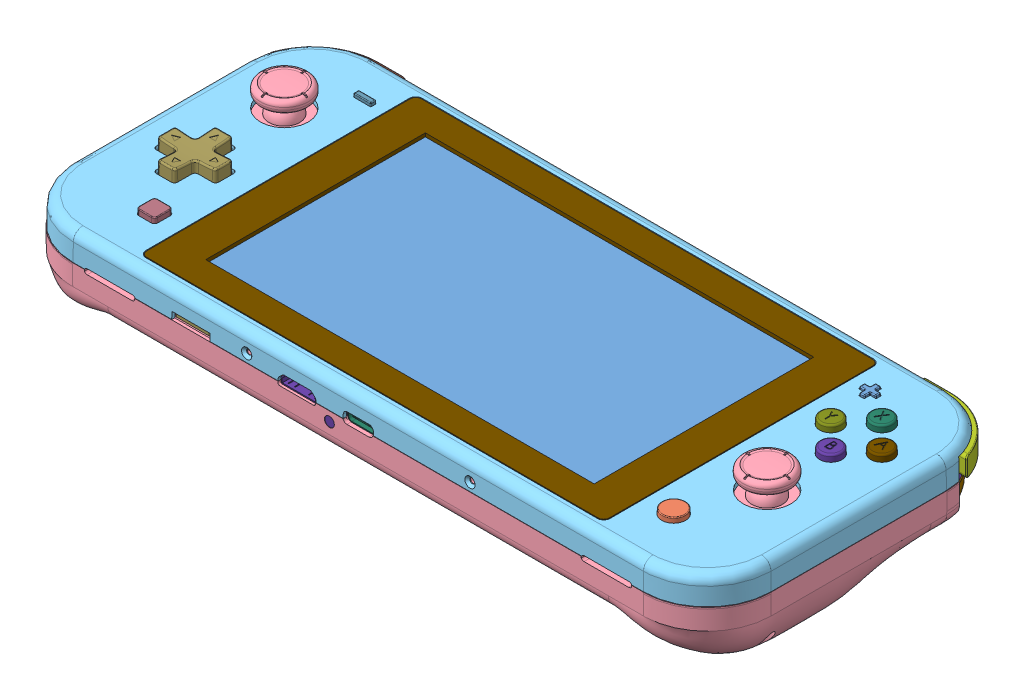
SolidWorks assembly Assembly Retro Lite CM5_1, configuration Default. Lengths in mm. (continued)
Components (placement in the parent): (continued)
- Switch Lite D-Pad_1-1: Switch Lite D-Pad_1 [Default] at (-86.4992 8.2269 18.5) size (20.6 9.05 20.6)
- Select_Button_1-1: Select_Button_1 [Default] at (-1.1992 10.6269 0) size (9.88 4.75 9.88)
- Minus Button_1-1: Minus Button_1 [Default] at (-93.2142 14.0269 -94.6231) x (0 0 -1) z (1 0 0) size (5.72 4.5 9.47)
- NuckDeck X_1-1: NuckDeck X_1 [Default] at (89.6642 6.7269 -27) size (9.68 5.75 9.89)
- NuckDeck Y_1-1: NuckDeck Y_1 [Default] at (81.6642 6.2269 -19) size (9.68 5.75 9.89)
- NuckDeck B_1-1: NuckDeck B_1 [Default] at (89.6642 6.7269 -11) size (9.68 5.75 9.89)
- NuckDeck A_1-1: NuckDeck A_1 [Default] at (97.6642 7.2269 -19) size (9.68 5.75 9.89)
- Plus_Button_1-1: Plus_Button_1 [Default] at (1.1992 9.5269 0) size (5.18 4.7 5.18)
- Start_Button_1-1: Start_Button_1 [Default] at (55.5311 21.0456 -12.0161) x (0 -1 0) z (0 0 1) size (5.05 11.38 11.38)
- Power-Volume Button-On_Off-1: Power-Volume Button-On_Off [Default] at (52.5142 1.7499 -46.5415) x (-1 0 0) z (0 -1 0) size (9.02 8.15 5.02)
- Switch Lite Fan_1-1: Switch Lite Fan_1 [Default] at (-39.8893 -3 21.8439) x (-1 0 0) z (0 0 1) size (44.11 7.2 36.36)
- Case Front_2-1: Case Front_2 [Default] at origin size (219.25 9 95.96)
- Volume Buttons-1: Volume Buttons [Default] at (0.7169 -0.25 -2.25) size (13.02 5.02 8.15)
- Cast Top Trigger Button_1-1: Cast Top Trigger Button_1 [Default] at (89.5015 1 -27.5865) size (30.55 6.25 18.5)
- Trigger Mount_1-1: Trigger Mount_1 [Default] at (89.5015 -0.5 -27.5865) size (33.8 9.9 32.8)
- ZR Trigger_1-1: ZR Trigger_1 [Default] at (89.5015 -9.2 -27.5865) size (28.44 13.7 22.93)
- MirrorZR Trigger_1-5: MirrorZR Trigger_1 [Default] at (-89.5015 -9.2 -27.5865) x (-1 0 0) z (0 0 -1) size (28.44 13.7 22.93)
- MirrorCast Top Trigger Button_1-4: MirrorCast Top Trigger Button_1 [Default] at (-89.5015 1 -27.5865) x (-1 0 0) z (0 0 -1) size (30.55 6.25 18.5)
- MirrorTrigger Mount_1-4: MirrorTrigger Mount_1 [Default] at (-89.5015 -0.5 -27.5865) x (-1 0 0) z (0 0 -1) size (33.8 9.9 32.8)
- Silicone Button Cap_ABXY-1: Silicone Button Cap_ABXY [Default] at (77.3642 2.35 -7) size (24.6 3.9 24)
- Silicone Button Cap_Circle-1: Silicone Button Cap_Circle [Default] at (77.0992 2.35 34) size (8.6 3.9 8)
- Silicone Button Cap_Square-1: Silicone Button Cap_Square [Default] at (-85.4948 2.75 33.8188) size (8.6 3.9 8)
- Silicone Button Cap_DPAD-1: Silicone Button Cap_DPAD [Default] at (-101.3932 2.75 20.344) size (23.6 3.9 23)
- VLP-350-F-1: VLP-350-F [Default] at (-6.6209 -4.3495 38.5774) x (0 0 1) z (-1 0 0) size (10.46 5.38 5.18)
- new battery-1: new battery [Default] at (8.52 -7.57 36.1416) size (55 11.5 71)
- battery bracket_3-1: battery bracket_3 [Default] at (39.5421 -1.57 -3.3584) size (64.54 12 77.4)
- fan bracket_2-1: fan bracket_2 [Default] at (-72.2632 -7.5 34.8151) size (61.54 7.08 37.55)
- battery bracket cover-1: battery bracket cover [Default] at (36.02 -8.37 0.6416) size (57.4 5.8 77.4)
- Case Rear_5-1: Case Rear_5 [Default] at (0 -9.5 0) size (221.26 27.07 96.31)
Mates (geometry in assembly coordinates):
- Width3: width anti-aligned: plane of Case Rear_1-1 through (-109.665 -9.5 47.5) normal (0 -0.008727 0.999962); plane of Case Rear_1-1 through (-109.665 -9.5 -47.5) normal (0 -0.008727 -0.999962); plane of Case Front_1-1 through (-109.665 0 -47.5) normal (0 0.008727 -0.999962); plane of Case Front_1-1 through (-109.665 0 47.5) normal (0 0.008727 0.999962)
- Width4: width anti-aligned: plane of Case Rear_1-1 through (109.665 -9.5 -47.5) normal (0.999962 -0.008727 0); plane of Case Rear_1-1 through (-109.665 -9.5 -47.5) normal (-0.999962 -0.008727 0); plane of Case Front_1-1 through (-109.665 0 -47.5) normal (-0.999962 0.008727 0); plane of Case Front_1-1 through (109.665 0 -47.5) normal (0.999962 0.008727 0)
- Coincident3: coincident anti-aligned: plane of Case Front_1-1 through (0 -1 0) normal (0 -1 0); plane of Case Rear_1-1 through (0 -1 0) normal (0 1 0)
- Width7: width: plane of Case Front_1-1 through (-88.8142 10.5 -0.8) normal (0 -0.008727 0.999962); plane of Case Front_1-1 through (-93.5142 10.5 18.8) normal (0 -0.008727 -0.999962); plane of Switch Lite D-Pad_1-1 through (-92.5892 8.2269 18.25) normal (0 0.034899 0.999391); plane of Switch Lite D-Pad_1-1 through (-86.7392 8.2269 -0.25) normal (0 0.034899 -0.999391)
- Coincident13: coincident anti-aligned: plane of Assembly Left PCB Controller-1/Single Silicone Cap-1 through (-79.0502 6.2769 -33.942) normal (0 1 0); plane of Minus Button_1-1 through (-79.0502 6.2769 -33.942) normal (0 -1 0)
- Parallel1: parallel aligned: plane of NuckDeck X_1-1 through (89.6642 6.7269 -27) normal (0 0 1)
- Parallel2: parallel aligned: plane of NuckDeck Y_1-1 through (81.6642 6.2269 -19) normal (0 0 1)
- Parallel3: parallel aligned: plane of NuckDeck B_1-1 through (89.6642 6.7269 -11) normal (0 0 1)
- Parallel4: parallel aligned: plane of NuckDeck A_1-1 through (97.6642 7.2269 -19) normal (0 0 1)
- Coincident21: coincident anti-aligned: plane of Assembly Right PCB Controller-1/Single Silicone Cap-2 through (79.0842 6.2769 -33.8353) normal (0 1 0); plane of Plus_Button_1-1 through (79.0842 6.2769 -33.8353) normal (0 -1 0)
- Parallel7: parallel aligned: plane of Start_Button_1-1 through (55.5311 21.0456 -12.0161) normal (0 0 1)
- Concentric10: concentric anti-aligned: cone of Case Front_1-1 through (52.675 2.9999 -45.4) axis (0 0 1); cone of Power-Volume Button-On_Off-1 through (52.675 1.9999 -46.0964) axis (0 0 -1)
- Parallel8: parallel anti-aligned: plane of Power-Volume Button-On_Off-1 through (52.5142 1.7499 -46.5415) normal (0 -1 0)
- Distance1: distance = 1 mm anti-aligned: plane of Assembly Center Components-1/Retro Lite CM5 (Latest)-18-1 through (46.5443 6.2108 -39.3999) normal (0 0 -1); plane of Power-Volume Button-On_Off-1 through (52.5142 1.7499 -40.3999) normal (0 0 1)
- Parallel9: parallel anti-aligned: plane of Power-Volume Button-Plus-1 through (41.7973 1.9999 -44.2915) normal (0 -1 0)
- Concentric12: concentric anti-aligned: cone of Case Front_1-1 through (33.5497 2.9999 -45.4) axis (0 0 1); cone of Power-Volume Button-Minus-1 through (33.5497 1.9999 -46.0964) axis (0 0 -1)
- Parallel10: parallel anti-aligned: plane of Power-Volume Button-Minus-1 through (33.3889 1.9999 -44.2915) normal (0 -1 0)
- Coincident24: coincident aligned: plane of Power-Volume Button-Plus-1 through (41.9582 1.9999 -41.4499) normal (0 0 1); plane of Power-Volume Button-Minus-1 through (33.5497 1.9999 -41.4499) normal (0 0 1)
- Parallel11: parallel aligned: plane of Assembly Left PCB Controller-1 through (-1.1992 8.75 0) normal (0 0 1)
- Coincident29: coincident anti-aligned: plane of Assembly Left PCB Controller-1/Switch Joystick Blank-2 through (-81.9642 8 -28) normal (0 1 0); plane of Case Front_2-1 through (0 8 0) normal (0 -1 0)
- Width17: width aligned: plane of Case Front_2-1 through (-99.4642 9.5 6.65) normal (0.999962 -0.008727 0); plane of Switch Lite D-Pad_1-1 through (-79.8642 9.5 6.65) normal (-0.999962 -0.008727 0); plane of Case Front_2-1 through (-80.4142 8.2269 11.925) normal (0.999391 0.034899 0); plane of Switch Lite D-Pad_1-1 through (-98.9142 8.2269 6.075) normal (-0.999391 0.034899 0)
- Width18: width anti-aligned: plane of Case Front_2-1 through (-92.0142 9.5 18.8) normal (0 -0.008727 -0.999962); plane of Switch Lite D-Pad_1-1 through (-87.3142 9.5 -0.8) normal (0 -0.008727 0.999962); plane of Case Front_2-1 through (-92.5892 8.2269 18.25) normal (0 0.034899 0.999391); plane of Switch Lite D-Pad_1-1 through (-86.7392 8.2269 -0.25) normal (0 0.034899 -0.999391)
- Width19: width aligned: plane of Minus Button_1-1 through (-76.7042 10.5269 -34.5841) normal (0 0.008727 -0.999962); plane of Case Front_2-1 through (-81.7042 10.5269 -32.9341) normal (0 0.008727 0.999962); plane of Minus Button_1-1 through (-81.7542 9.5 -32.8841) normal (0 -0.008727 -0.999962); plane of Case Front_2-1 through (-81.7542 9.5 -34.6341) normal (0 -0.008727 0.999962)
- Width20: width aligned: plane of Minus Button_1-1 through (-76.5042 10.5269 -33.1341) normal (0.999962 0.008727 0); plane of Case Front_2-1 through (-81.9042 10.5269 -34.3841) normal (-0.999962 0.008727 0); plane of Minus Button_1-1 through (-81.9542 9.5 -34.4341) normal (0.999962 -0.008727 0); plane of Case Front_2-1 through (-76.4542 9.5 -34.4341) normal (-0.999962 -0.008727 0)
- Width21: width aligned: plane of Select_Button_1-1 through (-78.4532 11.1269 28.1) normal (0.999962 0.008727 0); plane of Case Front_2-1 through (-84.2532 11.1269 28.1) normal (-0.999962 0.008727 0); plane of Select_Button_1-1 through (-84.3532 9.5 28) normal (0.999962 -0.008727 0); plane of Case Front_2-1 through (-78.3532 9.5 28) normal (-0.999962 -0.008727 0)
- Width22: width aligned: plane of Select_Button_1-1 through (-83.2532 11.1269 32.9) normal (0 0.008727 0.999962); plane of Case Front_2-1 through (-83.2532 11.1269 27.1) normal (0 0.008727 -0.999962); plane of Select_Button_1-1 through (-83.3532 9.5 27) normal (0 -0.008727 0.999962); plane of Case Front_2-1 through (-83.3532 9.5 33) normal (0 -0.008727 -0.999962)
- Concentric18: concentric aligned: circle of Assembly Left PCB Controller-1/Switch Joystick Blank-2; cone of Case Front_2-1 through (-89.6642 9.5 -19) axis (0 1 0)
- Concentric19: concentric aligned: circle of Assembly Right PCB Controller-1/Switch Joystick Blank-1; cone of Case Front_2-1 through (89.6642 9.5 9) axis (0 1 0)
- Width23: width anti-aligned: plane of Assembly Center Components-1/5.5_ Touch Display MIPI-1/CTP-1 through (-70.7372 9.5 -43.045) normal (0 0 -1); plane of Case Front_2-1 through (70.737 9.5 43.045) normal (0 0 1); plane of Assembly Center Components-1/5.5_ Touch Display MIPI-1/CTP-1 through (-70.737 8.4 43.295) normal (0 0.008727 -0.999962); plane of Case Front_2-1 through (70.737 8.4 -43.295) normal (0 0.008727 0.999962)
- Width24: width aligned: plane of Assembly Center Components-1/5.5_ Touch Display MIPI-1/CTP-1 through (72.505 9.5 -41.277) normal (1 0 0); plane of Case Front_2-1 through (-72.505 9.5 41.277) normal (-1 0 0); plane of Assembly Center Components-1/5.5_ Touch Display MIPI-1/CTP-1 through (72.755 8.4 41.277) normal (-0.999962 0.008727 0); plane of Case Front_2-1 through (-72.755 8.4 -41.277) normal (0.999962 0.008727 0)
- Coincident31: coincident anti-aligned: plane of Assembly Center Components-1/5.5_ Touch Display MIPI-1/CTP-1 through (0 8.4 0) normal (0 -1 0); plane of Case Front_2-1 through (-70.737 8.4 -41.277) normal (0 1 0)
- Concentric20: concentric anti-aligned: cone of Power-Volume Button-Plus-1 through (41.9582 1.9999 -46.0964) axis (0 0 -1); cone of Case Front_2-1 through (41.9582 1.9999 -43.4) axis (0 0 1)
- Parallel13: parallel aligned: plane of Assembly Right PCB Controller-1 through (1.1992 8.75 0) normal (0 0 1)
- Coincident32: coincident anti-aligned: plane of Assembly Right PCB Controller-1/Switch Joystick Blank-1 through (81.9642 8 18) normal (0 1 0); plane of Case Front_2-1 through (0 8 0) normal (0 -1 0)
- Concentric21: concentric aligned: cone of NuckDeck Y_1-1 through (81.6642 10.9531 -19) axis (0 1 0); cone of Case Front_2-1 through (81.6642 9.5 -19) axis (0 1 0)
- Concentric22: concentric aligned: cone of NuckDeck X_1-1 through (89.6642 10.9531 -27) axis (0 1 0); cone of Case Front_2-1 through (89.6642 9.5 -27) axis (0 1 0)
- Concentric23: concentric aligned: cone of NuckDeck A_1-1 through (97.6642 10.9531 -19) axis (0 1 0); cone of Case Front_2-1 through (97.6642 9.5 -19) axis (0 1 0)
- Concentric24: concentric aligned: cone of NuckDeck B_1-1 through (89.6642 10.9531 -11) axis (0 1 0); cone of Case Front_2-1 through (89.6642 9.5 -11) axis (0 1 0)
- Width25: width aligned: plane of Case Front_2-1 through (76.4542 9.5 -33.084) normal (0.999962 -0.008727 0); plane of Plus_Button_1-1 through (81.9542 9.5 -34.434) normal (-0.999962 -0.008727 0); plane of Case Front_2-1 through (81.7542 10.0256 -33.134) normal (0.999962 0.008727 0); plane of Plus_Button_1-1 through (76.6542 10.0256 -34.384) normal (-0.999962 0.008727 0)
- Width26: width aligned: plane of Case Front_2-1 through (78.5292 9.5 -36.509) normal (0 -0.008727 0.999962); plane of Plus_Button_1-1 through (79.8792 9.5 -31.009) normal (0 -0.008727 -0.999962); plane of Case Front_2-1 through (78.5792 10.0256 -31.209) normal (0 0.008727 0.999962); plane of Plus_Button_1-1 through (78.5792 10.0256 -36.309) normal (0 0.008727 -0.999962)
- Concentric25: concentric aligned: cone of Start_Button_1-1 through (81.3992 10.7269 30) axis (0 1 0); cone of Case Front_2-1 through (81.3992 9.5 30) axis (0 1 0)
- Concentric27: concentric anti-aligned: cone of Power-Volume Button-Minus-1 through (33.5497 1.9999 -46.0964) axis (0 0 -1); cone of Case Front_2-1 through (33.5497 1.9999 -43.4) axis (0 0 1)
- Concentric28: concentric anti-aligned: cone of Power-Volume Button-On_Off-1 through (52.675 1.7499 -44.6999) axis (0 0 -1); cone of Case Front_2-1 through (52.675 1.7499 -43.4) axis (0 0 1)
- Parallel15: parallel aligned: plane of Volume Buttons-1 through (0.7169 -0.25 -2.25) normal (0 1 0)
- Concentric31: concentric anti-aligned: cone of Case Front_2-1 through (42.675 1.7499 -43.4) axis (0 0 1); cone of Volume Buttons-1 through (42.675 1.7499 -49.7595) axis (0 0 -1)
- Coincident33: coincident aligned: plane of Power-Volume Button-On_Off-1 through (52.5142 1.7499 -40.3999) normal (0 0 1); plane of Volume Buttons-1 through (0.7169 -0.25 -40.3999) normal (0 0 1)
- Width27: width anti-aligned: plane of Case Front_2-1 through (-109.415 0 -47.5) normal (-0.999962 0.008727 0); plane of Case Rear_2-1 through (109.415 0 -47.5) normal (0.999962 0.008727 0); plane of Case Front_2-1 through (109.415 -9.5 -47.5) normal (0.999962 -0.008727 0); plane of Case Rear_2-1 through (-109.415 -9.5 -47.5) normal (-0.999962 -0.008727 0)
- Width28: width aligned: plane of Case Rear_2-1 through (-109.415 -9.5 47.5) normal (0 -0.008727 0.999962); plane of Case Front_2-1 through (-109.415 -9.5 -47.5) normal (0 -0.008727 -0.999962); plane of Case Rear_2-1 through (-109.415 0 47.5) normal (0 0.008727 0.999962); plane of Case Front_2-1 through (-109.415 0 -47.5) normal (0 0.008727 -0.999962)
- Coincident35: coincident anti-aligned: plane of Case Front_2-1 through (0 0.5 0) normal (0 -1 0); plane of Case Rear_2-1 through (0 0.5 0) normal (0 1 0)
- Width29: width aligned: plane of Case Rear_2-1 through (62.42 -7.5 39.75) normal (-0.999962 0.008727 0); plane of 855080 1s 4000mah-1 through (6.92 -7.5 -35.75) normal (0.999962 0.008727 0); plane of Case Rear_2-1 through (59.17 1 45.5) normal (1 0 0); plane of 855080 1s 4000mah-1 through (9.17 1 45.5) normal (-1 0 0)
- Width30: width anti-aligned: plane of 855080 1s 4000mah-1 through (59.17 1 45.5) normal (0 0 1); plane of Case Rear_2-1 through (59.17 1 -34.5) normal (0 0 -1); plane of 855080 1s 4000mah-1 through (62.42 -7.5 -35.75) normal (0 0.008727 0.999962); plane of Case Rear_2-1 through (6.92 -7.5 39.75) normal (0 0.008727 -0.999962)
- Coincident36: coincident anti-aligned: plane of 855080 1s 4000mah-1 through (59.17 -7.5 45.5) normal (0 -1 0); plane of Case Rear_2-1 through (0 -7.5 0) normal (0 1 0)
- Coincident40: coincident aligned: plane of Case Rear_2-1 through (89.5015 1 27.5865) normal (0 1 0); plane of Trigger Mount_1-1 through (89.5015 1 -27.5865) normal (0 1 0)
- Concentric37: concentric anti-aligned: cylinder of Trigger Mount_1-1 through (89.5015 1 -27.5865) axis (0 -1 0) radius 17.8007
- Parallel17: parallel aligned: plane of Trigger Mount_1-1 through (89.5015 -0.5 -27.5865) normal (0 0 1)
- Parallel18: parallel aligned: plane of Cast Top Trigger Button_1-1 through (89.5015 1 -27.5865) normal (0 0 1)
- Coincident41: coincident anti-aligned: plane of Cast Top Trigger Button_1-1 through (89.5015 1 -27.5865) normal (0 -1 0); plane of Trigger Mount_1-1 through (89.5015 1 -27.5865) normal (0 1 0)
- Parallel19: parallel aligned: plane of ZR Trigger_1-1 through (89.5015 -9.2 -27.5865) normal (0 0 1)
- Concentric41: concentric aligned: cylinder of Trigger Mount_1-1 through (89.5015 1 -27.5865) axis (0 -1 0) radius 17.8007; cylinder of ZR Trigger_1-1 through (89.5015 -2.9 -27.5865) axis (0 -1 0) radius 18.0007
- Distance2: distance = 0.9 mm anti-aligned: plane of ZR Trigger_1-1 through (89.5015 -2.4 -27.5865) normal (0 1 0); plane of Trigger Mount_1-1 through (94.8858 -2.2 -27.3249) normal (0 -1 0)
- Coincident43: coincident anti-aligned: plane of Case Rear_2-1 through (0 -7.5 0) normal (0 1 0); plane of 5000mah battery-1 through (34.67 -7.5 2) normal (0 -1 0)
- Concentric43: concentric aligned: cone of Battery Bracket-1 through (65.42 -5.5 11.5) axis (0 -1 0); cone of Case Rear_2-1 through (65.92 -7.5 8) axis (0 -1 0)
- Coincident44: coincident anti-aligned: plane of Battery Bracket-1 through (65.42 -5.5 11.5) normal (0 -1 0); plane of Case Rear_2-1 through (0 -5.5 0) normal (0 1 0)
- Concentric46: concentric aligned: cone of NuckDeck X_1-1 through (89.6642 10.9531 -27) axis (0 1 0); circle of Silicone Button Cap_ABXY-1
- Concentric47: concentric aligned: cone of NuckDeck B_1-1 through (89.6642 10.9531 -11) axis (0 1 0); circle of Silicone Button Cap_ABXY-1
- Coincident48: coincident anti-aligned: plane of Assembly Right PCB Controller-1/Retrolite CM5 RCPCB v1 - RP2040 v2-1/Board (39)-1 through (86.1244 2.35 -1.5702) normal (0 1 0); plane of Silicone Button Cap_ABXY-1 through (77.3642 2.35 -7) normal (0 -1 0)
- Concentric48: concentric anti-aligned: cone of Start_Button_1-1 through (81.3992 10.7269 30) axis (0 1 0); circle of Silicone Button Cap_Circle-1
- Parallel20: parallel aligned: plane of Silicone Button Cap_Circle-1 through (77.0992 4.55 34) normal (0 0 1)
- Coincident49: coincident anti-aligned: plane of Assembly Right PCB Controller-1/Retrolite CM5 RCPCB v1 - RP2040 v2-1/Board (39)-1 through (86.1244 2.35 -1.5702) normal (0 1 0); plane of Silicone Button Cap_Circle-1 through (77.0992 2.35 34) normal (0 -1 0)
- Concentric49: concentric aligned: cylinder of Assembly Left PCB Controller-1/Retro Lite CM5 (Latest)-10-1 through (-81.1948 12.0195 29.8188) axis (0 -1 0) radius 1.5; circle of Silicone Button Cap_Square-1
- Parallel21: parallel aligned: plane of Silicone Button Cap_Square-1 through (-85.4948 4.95 33.8188) normal (0 0 1)
- Coincident50: coincident anti-aligned: plane of Assembly Left PCB Controller-1/Retrolite CM5 LCPCB v2 v1 (4)-1/Board (38)-1 through (-88.9703 2.75 -1.3591) normal (0 1 0); plane of Silicone Button Cap_Square-1 through (-85.4948 2.75 33.8188) normal (0 -1 0)
- Concentric50: concentric anti-aligned: cylinder of Assembly Left PCB Controller-1/Retro Lite CM5 (Latest)-1 through (-89.5932 12.0195 1.344) axis (0 -1 0) radius 1.5; circle of Silicone Button Cap_DPAD-1
- Parallel22: parallel anti-aligned: plane of Silicone Button Cap_DPAD-1 through (-101.3932 4.95 20.344) normal (-1 0 0)
- Coincident51: coincident anti-aligned: plane of Assembly Left PCB Controller-1/Retrolite CM5 LCPCB v2 v1 (4)-1/Board (38)-1 through (-88.9703 2.75 -1.3591) normal (0 1 0); plane of Silicone Button Cap_DPAD-1 through (-101.3932 2.75 20.344) normal (0 -1 0)
- Coincident52: coincident anti-aligned: plane of Select_Button_1-1 through (-81.3532 6.65 30) normal (0 -1 0); plane of Silicone Button Cap_Square-1 through (-81.1948 6.65 29.8188) normal (0 1 0)
- Coincident53: coincident anti-aligned: plane of Switch Lite D-Pad_1-1 through (-89.6642 6.65 18.3704) normal (0 -1 0); plane of Silicone Button Cap_DPAD-1 through (-89.5932 6.65 16.344) normal (0 1 0)
- Coincident54: coincident anti-aligned: plane of NuckDeck A_1-1 through (95.9498 6.25 -19) normal (0 -1 0); plane of Silicone Button Cap_ABXY-1 through (97.6642 6.25 -19) normal (0 1 0)
- Coincident55: coincident anti-aligned: plane of NuckDeck X_1-1 through (87.9498 6.25 -27) normal (0 -1 0); plane of Silicone Button Cap_ABXY-1 through (89.6642 6.25 -27) normal (0 1 0)
- Coincident56: coincident anti-aligned: plane of NuckDeck Y_1-1 through (79.9498 6.25 -19) normal (0 -1 0); plane of Silicone Button Cap_ABXY-1 through (81.6642 6.25 -19) normal (0 1 0)
- Coincident57: coincident anti-aligned: plane of NuckDeck B_1-1 through (87.9498 6.25 -11) normal (0 -1 0); plane of Silicone Button Cap_ABXY-1 through (89.6642 6.25 -11) normal (0 1 0)
- Coincident58: coincident anti-aligned: plane of Start_Button_1-1 through (83.1136 6.25 30) normal (0 -1 0); plane of Silicone Button Cap_Circle-1 through (81.3992 6.25 30) normal (0 1 0)
- Concentric51: concentric anti-aligned: cone of Case Rear_2-1 through (-8.9704 -2 42.5) axis (0 0 -1); circle of VLP-350-F-1
- Parallel23: parallel aligned: plane of VLP-350-F-1 through (-6.6209 -4.3495 38.5774) normal (0 1 0)
- Coincident59: coincident anti-aligned: plane of Case Rear_2-1 through (0 -7.5 0) normal (0 1 0); plane of 6000mah battery-1 through (8.92 -7.5 40.3584) normal (0 -1 0)
- Width31: width aligned: plane of 6000mah battery-1 through (7.92 4.9 -40.6416) normal (0 0 -1); plane of Case Rear_2-1 through (65.92 4.9 44.3584) normal (0 0 1); plane of 6000mah battery-1 through (64.12 -7.5 -33.3416) normal (0 0.008727 0.999962); plane of Case Rear_2-1 through (8.72 -7.5 38.0584) normal (0 0.008727 -0.999962)
- Width32: width anti-aligned: plane of 6000mah battery-1 through (7.92 4.9 44.3584) normal (-1 0 0); plane of Case Rear_2-1 through (65.92 4.9 -40.6416) normal (1 0 0); plane of 6000mah battery-1 through (64.12 -7.5 38.0584) normal (-0.999962 0.008727 0); plane of Case Rear_2-1 through (8.72 -7.5 -33.3416) normal (0.999962 0.008727 0)
- Parallel24: parallel aligned: plane of Battery Bracket_1-1 through (25.32 -6.5 2.5234) normal (1 0 0)
- Concentric53: concentric aligned: cylinder of Assembly Left PCB Controller-1/Retrolite CM5 LCPCB v2 v1 (4)-1/Board (38)-1 through (-73.7632 11.08 34.8151) axis (0 -1 0) radius 1; cone of fan bracket-1 through (-73.7632 -7.5 34.8151) axis (0 -1 0)
- Concentric54: concentric aligned: cylinder of Assembly Left PCB Controller-1/Retrolite CM5 LCPCB v2 v1 (4)-1/Board (38)-1 through (-73.7632 11.08 24.8151) axis (0 -1 0) radius 1; cone of fan bracket-1 through (-73.7632 -7.5 24.8151) axis (0 -1 0)
- Coincident61: coincident anti-aligned: plane of Assembly Left PCB Controller-1/Retrolite CM5 LCPCB v2 v1 (4)-1/Board (38)-1 through (-88.9703 1.08 -1.3591) normal (0 -1 0); plane of fan bracket-1 through (-32.306 1.08 24.969) normal (0 1 0)
- Concentric55: concentric anti-aligned: cylinder of Assembly Right PCB Controller-1/Retrolite CM5 RCPCB v1 - RP2040 v2-1/Board (39)-1 through (69.3642 0.68 -31) axis (0 1 0) radius 1; cylinder of battery bracket_3-1 through (69.3642 3.43 -31) axis (0 -1 0) radius 1
- Concentric56: concentric anti-aligned: cylinder of Assembly Right PCB Controller-1/Retrolite CM5 RCPCB v1 - RP2040 v2-1/Board (39)-1 through (69.3642 0.68 30) axis (0 1 0) radius 1; cylinder of battery bracket_3-1 through (69.3642 3.43 30) axis (0 -1 0) radius 1
- Coincident62: coincident anti-aligned: plane of Assembly Right PCB Controller-1/Retrolite CM5 RCPCB v1 - RP2040 v2-1/Board (39)-1 through (86.1244 0.68 -1.5702) normal (0 -1 0); plane of battery bracket_3-1 through (65.62 0.68 -73) normal (0 1 0)
- Width33: width aligned: plane of battery bracket_3-1 through (64.12 3.43 -35.0584) normal (0 0 1); plane of battery bracket_3-1 through (8.72 3.43 36.3416) normal (0 0 -1); plane of new battery-1 through (63.52 3.93 36.1416) normal (0 0 1); plane of new battery-1 through (8.52 3.93 -34.8584) normal (0 0 -1)
- Width34: width aligned: plane of battery bracket_3-1 through (8.32 3.43 -39.0584) normal (1 0 0); plane of battery bracket_3-1 through (63.72 3.43 32.3416) normal (-1 0 0); plane of new battery-1 through (63.52 3.93 -34.8584) normal (1 0 0); plane of new battery-1 through (8.52 3.93 36.1416) normal (-1 0 0)
- Concentric57: concentric aligned: cylinder of Assembly Left PCB Controller-1/Retrolite CM5 LCPCB v2 v1 (4)-1/Board (38)-1 through (-73.7632 11.08 34.8151) axis (0 -1 0) radius 1; cone of fan bracket_2-1 through (-73.7632 -7.5 34.8151) axis (0 -1 0)
- Concentric58: concentric aligned: cylinder of Assembly Left PCB Controller-1/Retrolite CM5 LCPCB v2 v1 (4)-1/Board (38)-1 through (-73.7632 11.08 24.8151) axis (0 -1 0) radius 1; cone of fan bracket_2-1 through (-73.7632 -7.5 24.8151) axis (0 -1 0)
- Coincident64: coincident anti-aligned: plane of Assembly Left PCB Controller-1/Retrolite CM5 LCPCB v2 v1 (4)-1/Board (38)-1 through (-88.9703 1.08 -1.3591) normal (0 -1 0); plane of fan bracket_2-1 through (-56.0433 1.08 36.0396) normal (0 1 0)
- Concentric59: concentric anti-aligned: cylinder of Switch Lite Fan_1-1 through (-56.0433 -6 36.0396) axis (0 1 0) radius 1.6; cone of fan bracket_2-1 through (-56.0433 -7.5 36.0396) axis (0 -1 0)
- Concentric60: concentric anti-aligned: cylinder of Switch Lite Fan_1-1 through (-56.7839 -6 11.0668) axis (0 1 0) radius 1.6; cone of fan bracket_2-1 through (-56.7839 -7.5 11.0668) axis (0 -1 0)
- Coincident65: coincident anti-aligned: plane of Switch Lite Fan_1-1 through (-40.8723 -4.5 23.2357) normal (0 -1 0); plane of fan bracket_2-1 through (-64.1236 -4.5 56.8151) normal (0 1 0)
- Coincident66: coincident anti-aligned: plane of new battery-1 through (8.52 3.93 36.1416) normal (0 1 0); plane of battery bracket_3-1 through (39.5421 3.93 -3.3584) normal (0 -1 0)
- Coincident67: coincident aligned: plane of battery bracket_3-1 through (65.62 3.43 -38.0584) normal (0 0 -1); plane of battery bracket cover-1 through (7.32 -7.57 -38.0584) normal (0 0 -1)
- Coincident68: coincident aligned: plane of battery bracket_3-1 through (64.72 3.43 33.8416) normal (1 0 0); plane of battery bracket cover-1 through (64.72 -7.57 -38.0584) normal (1 0 0)
- Coincident69: coincident anti-aligned: plane of battery bracket_3-1 through (39.5421 -7.57 -3.3584) normal (0 -1 0); plane of battery bracket cover-1 through (36.02 -7.57 0.6416) normal (0 1 0)
- Concentric61: concentric anti-aligned: cone of Case Front_2-1 through (-69.5015 7.5 -43.4016) axis (0 1 0); cone of Case Rear_5-1 through (-69.5015 -7.5 -43.4016) axis (0 -1 0)
- Concentric62: concentric anti-aligned: cone of Case Front_2-1 through (69.5015 7.5 -43.4016) axis (0 1 0); cone of Case Rear_5-1 through (69.5015 -7.5 -43.4016) axis (0 -1 0)
- Coincident70: coincident anti-aligned: plane of Case Front_2-1 through (0 0.5 0) normal (0 -1 0); plane of Case Rear_5-1 through (0 0.5 0) normal (0 1 0)
